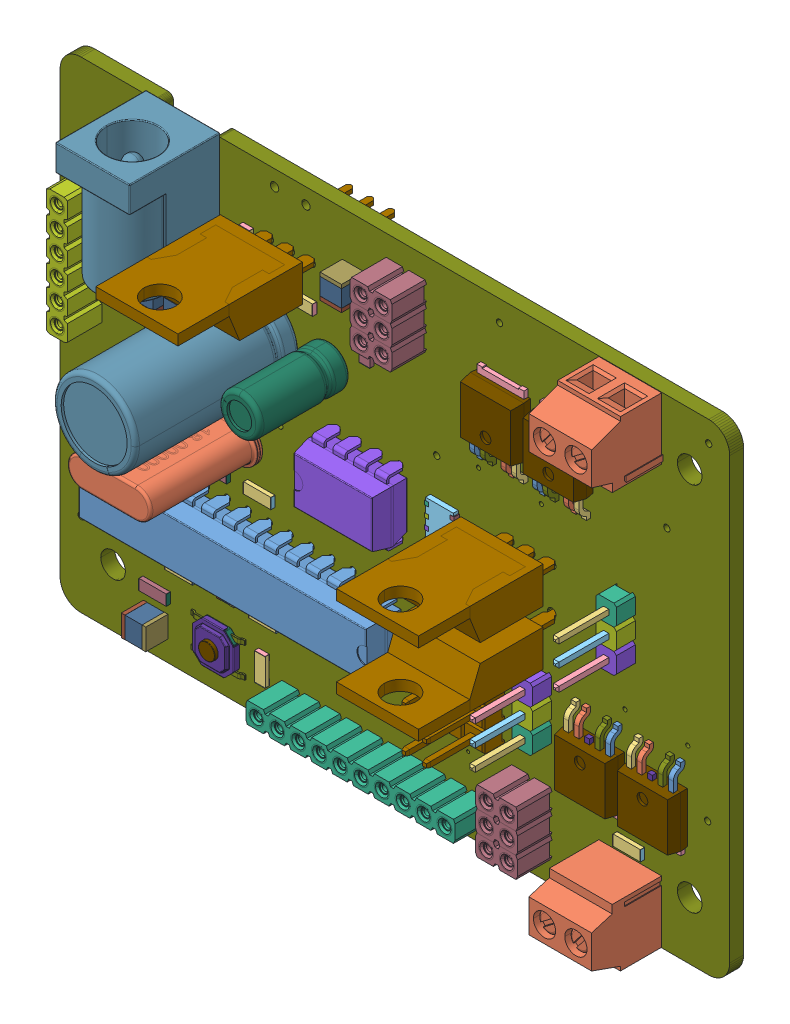
SolidWorks assembly Scheme_ver2, configuration По умолчанию. Lengths in mm.
Overall size (81.28 59.4 30.01).
257 component instances, 52 part files, 0 mates.
Components (placement in the parent):
- Scheme_ver2.STEP-1: Scheme_ver2.STEP [По умолчанию] at origin size (81.28 59.4 30.01)
  - U1.STEP-1: U1.STEP [По умолчанию] at (29.21 20.955 0.8452) x (-1 0 0) z (0 0 1) size (35.56 7.92 7.75)
    - Open CASCADE STEP translator 6.8 2.2.1.STEP-1: Open CASCADE STEP translator 6.8 2.2.1.STEP [По умолчанию] at origin size (35.56 7.92 7.75)
      - Body_1.STEP-1: Body_1.STEP [По умолчанию] at (16.5 3.8 0) x (0 1 0) z (1 0 0) size (7.92 7.75 35.56)
  - Y1.STEP-1: Y1.STEP [По умолчанию] at (10.16 27.94 0.8452) x (-1 0 0) z (0 0 1) size (11 4.5 15.2)
    - Open CASCADE STEP translator 6.8 2.3.1.STEP-1: Open CASCADE STEP translator 6.8 2.3.1.STEP [По умолчанию] at origin size (11 4.5 15.2)
      - Body_1-0.STEP-1: Body_1-0.STEP [По умолчанию] at (2.5 0 0) x (1 0 0) z (0 -1 0) size (11 15.2 4.5)
  - C6.STEP-1: C6.STEP [По умолчанию] at (6.35 31.7754 0.8452) x (0 1 0) z (0 0 1) size (3.35 1.3 0.55)
    - Open CASCADE STEP translator 6.8 2.4.1.STEP-1: Open CASCADE STEP translator 6.8 2.4.1.STEP [По умолчанию] at origin size (3.35 1.3 0.55)
      - Body_1-1.STEP-1: Body_1-1.STEP [По умолчанию] at origin size (3.3 1.3 0.48)
      - Pin_1.STEP-1: Pin_1.STEP [По умолчанию] at (0.5588 0 0) x (-1 0 0) z (0 0 1) size (0.76 1.27 0.55)
      - Pin_2.STEP-1: Pin_2.STEP [По умолчанию] at origin size (0.76 1.27 0.55)
  - C7.STEP-1: C7.STEP [По умолчанию] at (8.89 31.7754 0.8452) x (0 1 0) z (0 0 1) size (3.35 1.3 0.55)
    - Open CASCADE STEP translator 6.8 2.4.1.STEP-1: Open CASCADE STEP translator 6.8 2.4.1.STEP [По умолчанию] at origin size (3.35 1.3 0.55)
      - Body_1-1.STEP-1: Body_1-1.STEP [По умолчанию] at origin size (3.3 1.3 0.48)
      - Pin_1.STEP-1: Pin_1.STEP [По умолчанию] at (0.5588 0 0) x (-1 0 0) z (0 0 1) size (0.76 1.27 0.55)
      - Pin_2.STEP-1: Pin_2.STEP [По умолчанию] at origin size (0.76 1.27 0.55)
  - J1.STEP-1: J1.STEP [По умолчанию] at (16.51 3.81 0.8452) size (25.4 2.54 7.37)
    - Open CASCADE STEP translator 6.8 2.6.1.STEP-1: Open CASCADE STEP translator 6.8 2.6.1.STEP [По умолчанию] at origin size (25.4 2.54 7.37)
      - Body_1-2.STEP-1: Body_1-2.STEP [По умолчанию] at (11.5 0 0) x (1 0 0) z (0 -1 0) size (25.4 7.37 2.54)
  - J2.STEP-1: J2.STEP [По умолчанию] at (-7.62 45.72 0.8452) x (0 -1 0) z (0 0 1) size (15.24 2.54 7.37)
    - Open CASCADE STEP translator 6.8 2.7.1.STEP-1: Open CASCADE STEP translator 6.8 2.7.1.STEP [По умолчанию] at origin size (15.24 2.54 7.37)
      - Body_1-3.STEP-1: Body_1-3.STEP [По умолчанию] at (6.5 0 0) x (1 0 0) z (0 -1 0) size (15.24 7.37 2.54)
  - U2.STEP-1: U2.STEP [По умолчанию] at (22.225 27.305 0.8452) size (10.16 7.92 7.75)
    - Open CASCADE STEP translator 6.8 2.8.1.STEP-1: Open CASCADE STEP translator 6.8 2.8.1.STEP [По умолчанию] at origin size (10.16 7.92 7.75)
      - Body_1-4.STEP-1: Body_1-4.STEP [По умолчанию] at (3.9 4 0) x (0 1 0) z (1 0 0) size (7.92 7.75 10.16)
  - VT1.STEP-1: VT1.STEP [По умолчанию] at (45.72 33.655 0.8452) size (9.97 4.45 28.62)
    - Open CASCADE STEP translator 6.8 2.9.1.STEP-1: Open CASCADE STEP translator 6.8 2.9.1.STEP [По умолчанию] at origin size (9.97 4.45 28.62)
      - Body_1-5.STEP-1: Body_1-5.STEP [По умолчанию] at (0 3 3.5) x (1 0 0) z (0 -1 0) size (9.97 28.62 4.45)
  - VT2.STEP-1: VT2.STEP [По умолчанию] at (45.72 28.575 0.8452) x (-1 0 0) z (0 0 1) size (9.97 4.45 28.62)
    - Open CASCADE STEP translator 6.8 2.10.1.STEP-1: Open CASCADE STEP translator 6.8 2.10.1.STEP [По умолчанию] at origin size (9.97 4.45 28.62)
      - Body_1-5.STEP-1: Body_1-5.STEP [По умолчанию] at (0 3 3.5) x (1 0 0) z (0 -1 0) size (9.97 28.62 4.45)
  - D2.STEP-1: D2.STEP [По умолчанию] at (1.63 3.81 0.8452) x (-1 0 0) z (0 0 1) size (2.97 2.6 2.7)
    - Open CASCADE STEP translator 6.8 2.11.1.STEP-1: Open CASCADE STEP translator 6.8 2.11.1.STEP [По умолчанию] at origin size (2.97 2.6 2.7)
      - Body_1-6.STEP-1: Body_1-6.STEP [По умолчанию] at origin size (2.6 2.58 2.68)
      - Pin_1-7.STEP-1: Pin_1-7.STEP [По умолчанию] at origin size (0.45 2.6 2.7)
      - Pin_2-8.STEP-1: Pin_2-8.STEP [По умолчанию] at (0.376 0 0) x (-1 0 0) z (0 0 1) size (0.45 2.6 2.7)
  - R3.STEP-1: R3.STEP [По умолчанию] at (-1.27 6.985 0.8452) size (3.35 1.3 0.55)
    - Open CASCADE STEP translator 6.8 2.12.1.STEP-1: Open CASCADE STEP translator 6.8 2.12.1.STEP [По умолчанию] at origin size (3.35 1.3 0.55)
      - Body_1-9.STEP-1: Body_1-9.STEP [По умолчанию] at origin size (3.3 1.3 0.48)
      - Pin_1-10.STEP-1: Pin_1-10.STEP [По умолчанию] at (0.5588 0 0) x (-1 0 0) z (0 0 1) size (0.76 1.27 0.55)
      - Pin_2-11.STEP-1: Pin_2-11.STEP [По умолчанию] at origin size (0.76 1.27 0.55)
  - C2.STEP-1: C2.STEP [По умолчанию] at (11.43 50.8 0.8452) x (0 -1 0) z (0 0 1) size (3.35 1.3 0.55)
    - Open CASCADE STEP translator 6.8 2.4.1.STEP-1: Open CASCADE STEP translator 6.8 2.4.1.STEP [По умолчанию] at origin size (3.35 1.3 0.55)
      - Body_1-1.STEP-1: Body_1-1.STEP [По умолчанию] at origin size (3.3 1.3 0.48)
      - Pin_1.STEP-1: Pin_1.STEP [По умолчанию] at (0.5588 0 0) x (-1 0 0) z (0 0 1) size (0.76 1.27 0.55)
      - Pin_2.STEP-1: Pin_2.STEP [По умолчанию] at origin size (0.76 1.27 0.55)
  - DA1.STEP-1: DA1.STEP [По умолчанию] at (16.51 50.8 0.8452) size (9.97 4.45 28.62)
    - Open CASCADE STEP translator 6.8 2.14.1.STEP-1: Open CASCADE STEP translator 6.8 2.14.1.STEP [По умолчанию] at origin size (9.97 4.45 28.62)
      - Body_1-5.STEP-1: Body_1-5.STEP [По умолчанию] at (0 3 3.5) x (1 0 0) z (0 -1 0) size (9.97 28.62 4.45)
  - C3.STEP-1: C3.STEP [По умолчанию] at (19.644 46.355 0.8452) x (-1 0 0) z (0 0 1) size (3.35 1.3 0.55)
    - Open CASCADE STEP translator 6.8 2.4.1.STEP-1: Open CASCADE STEP translator 6.8 2.4.1.STEP [По умолчанию] at origin size (3.35 1.3 0.55)
      - Body_1-1.STEP-1: Body_1-1.STEP [По умолчанию] at origin size (3.3 1.3 0.48)
      - Pin_1.STEP-1: Pin_1.STEP [По умолчанию] at (0.5588 0 0) x (-1 0 0) z (0 0 1) size (0.76 1.27 0.55)
      - Pin_2.STEP-1: Pin_2.STEP [По умолчанию] at origin size (0.76 1.27 0.55)
  - C5.STEP-1: C5.STEP [По умолчанию] at (11.43 23.495 0.8452) size (3.35 1.3 0.55)
    - Open CASCADE STEP translator 6.8 2.4.1.STEP-1: Open CASCADE STEP translator 6.8 2.4.1.STEP [По умолчанию] at origin size (3.35 1.3 0.55)
      - Body_1-1.STEP-1: Body_1-1.STEP [По умолчанию] at origin size (3.3 1.3 0.48)
      - Pin_1.STEP-1: Pin_1.STEP [По умолчанию] at (0.5588 0 0) x (-1 0 0) z (0 0 1) size (0.76 1.27 0.55)
      - Pin_2.STEP-1: Pin_2.STEP [По умолчанию] at origin size (0.76 1.27 0.55)
  - Q2.STEP-1: Q2.STEP [По умолчанию] at (39.9815 41.3198 0.8452) size (6.5 9.8 2.31)
    - Open CASCADE STEP translator 6.8 2.17.1.STEP-1: Open CASCADE STEP translator 6.8 2.17.1.STEP [По умолчанию] at origin size (6.5 9.8 2.31)
      - Body_1-12.STEP-1: Body_1-12.STEP [По умолчанию] at (2.4 5.35 0) size (6.5 9.8 2.31)
        - Scheme_ver2-prt15.STEP-1: Scheme_ver2-prt15.STEP [По умолчанию] at origin size (0.6 3 1.4)
        - Scheme_ver2-prt16.STEP-1: Scheme_ver2-prt16.STEP [По умолчанию] at (0.13 0 0) size (0.6 0.85 0.5)
        - Scheme_ver2-prt17.STEP-1: Scheme_ver2-prt17.STEP [По умолчанию] at (0.129 0.01 -0.0028) x (0.999999 0 -0.001062) z (0.001062 0 0.999999) size (6.5 6.22 2.3)
        - Scheme_ver2-prt18.STEP-1: Scheme_ver2-prt18.STEP [По умолчанию] at (-0.13 0 0) size (0.6 3 1.4)
        - Scheme_ver2-prt19.STEP-1: Scheme_ver2-prt19.STEP [По умолчанию] at (0.26 0 0) size (0.6 3 1.4)
        - Scheme_ver2-prt20.STEP-1: Scheme_ver2-prt20.STEP [По умолчанию] at (0.39 0 0) size (0.6 3 1.4)
        - Scheme_ver2-prt21.STEP-1: Scheme_ver2-prt21.STEP [По умолчанию] at (0.129 -0.1 -0.0028) x (0.999999 0 -0.001062) z (0.001062 0 0.999999) size (5.7 5.2 0.5)
  - Q1.STEP-1: Q1.STEP [По умолчанию] at (47.6015 41.3198 0.8452) size (6.5 9.8 2.31)
    - Open CASCADE STEP translator 6.8 2.18.1.STEP-1: Open CASCADE STEP translator 6.8 2.18.1.STEP [По умолчанию] at origin size (6.5 9.8 2.31)
      - Body_1-12.STEP-1: Body_1-12.STEP [По умолчанию] at (2.4 5.35 0) size (6.5 9.8 2.31)
        - Scheme_ver2-prt15.STEP-1: Scheme_ver2-prt15.STEP [По умолчанию] at origin size (0.6 3 1.4)
        - Scheme_ver2-prt16.STEP-1: Scheme_ver2-prt16.STEP [По умолчанию] at (0.13 0 0) size (0.6 0.85 0.5)
        - Scheme_ver2-prt17.STEP-1: Scheme_ver2-prt17.STEP [По умолчанию] at (0.129 0.01 -0.0028) x (0.999999 0 -0.001062) z (0.001062 0 0.999999) size (6.5 6.22 2.3)
        - Scheme_ver2-prt18.STEP-1: Scheme_ver2-prt18.STEP [По умолчанию] at (-0.13 0 0) size (0.6 3 1.4)
        - Scheme_ver2-prt19.STEP-1: Scheme_ver2-prt19.STEP [По умолчанию] at (0.26 0 0) size (0.6 3 1.4)
        - Scheme_ver2-prt20.STEP-1: Scheme_ver2-prt20.STEP [По умолчанию] at (0.39 0 0) size (0.6 3 1.4)
        - Scheme_ver2-prt21.STEP-1: Scheme_ver2-prt21.STEP [По умолчанию] at (0.129 -0.1 -0.0028) x (0.999999 0 -0.001062) z (0.001062 0 0.999999) size (5.7 5.2 0.5)
  - D1.STEP-1: D1.STEP [По умолчанию] at (24.13 52.98 0.8452) x (0 -1 0) z (0 0 1) size (2.97 2.6 2.7)
    - Open CASCADE STEP translator 6.8 2.11.1.STEP-1: Open CASCADE STEP translator 6.8 2.11.1.STEP [По умолчанию] at origin size (2.97 2.6 2.7)
      - Body_1-6.STEP-1: Body_1-6.STEP [По умолчанию] at origin size (2.6 2.58 2.68)
      - Pin_1-7.STEP-1: Pin_1-7.STEP [По умолчанию] at origin size (0.45 2.6 2.7)
      - Pin_2-8.STEP-1: Pin_2-8.STEP [По умолчанию] at (0.376 0 0) x (-1 0 0) z (0 0 1) size (0.45 2.6 2.7)
  - R1.STEP-1: R1.STEP [По умолчанию] at (26.035 43.815 0.8452) x (0 1 0) z (0 0 1) size (3.35 1.3 0.55)
    - Open CASCADE STEP translator 6.8 2.12.1.STEP-1: Open CASCADE STEP translator 6.8 2.12.1.STEP [По умолчанию] at origin size (3.35 1.3 0.55)
      - Body_1-9.STEP-1: Body_1-9.STEP [По умолчанию] at origin size (3.3 1.3 0.48)
      - Pin_1-10.STEP-1: Pin_1-10.STEP [По умолчанию] at (0.5588 0 0) x (-1 0 0) z (0 0 1) size (0.76 1.27 0.55)
      - Pin_2-11.STEP-1: Pin_2-11.STEP [По умолчанию] at origin size (0.76 1.27 0.55)
  - Q4.STEP-1: Q4.STEP [По умолчанию] at (64.095 20.67 0.8452) x (-1 0 0) z (0 0 1) size (6.5 9.8 2.31)
    - Open CASCADE STEP translator 6.8 2.21.1.STEP-1: Open CASCADE STEP translator 6.8 2.21.1.STEP [По умолчанию] at origin size (6.5 9.8 2.31)
      - Body_1-12.STEP-1: Body_1-12.STEP [По умолчанию] at (2.4 5.35 0) size (6.5 9.8 2.31)
        - Scheme_ver2-prt15.STEP-1: Scheme_ver2-prt15.STEP [По умолчанию] at origin size (0.6 3 1.4)
        - Scheme_ver2-prt16.STEP-1: Scheme_ver2-prt16.STEP [По умолчанию] at (0.13 0 0) size (0.6 0.85 0.5)
        - Scheme_ver2-prt17.STEP-1: Scheme_ver2-prt17.STEP [По умолчанию] at (0.129 0.01 -0.0028) x (0.999999 0 -0.001062) z (0.001062 0 0.999999) size (6.5 6.22 2.3)
        - Scheme_ver2-prt18.STEP-1: Scheme_ver2-prt18.STEP [По умолчанию] at (-0.13 0 0) size (0.6 3 1.4)
        - Scheme_ver2-prt19.STEP-1: Scheme_ver2-prt19.STEP [По умолчанию] at (0.26 0 0) size (0.6 3 1.4)
        - Scheme_ver2-prt20.STEP-1: Scheme_ver2-prt20.STEP [По умолчанию] at (0.39 0 0) size (0.6 3 1.4)
        - Scheme_ver2-prt21.STEP-1: Scheme_ver2-prt21.STEP [По умолчанию] at (0.129 -0.1 -0.0028) x (0.999999 0 -0.001062) z (0.001062 0 0.999999) size (5.7 5.2 0.5)
  - Q3.STEP-1: Q3.STEP [По умолчанию] at (56.475 20.67 0.8452) x (-1 0 0) z (0 0 1) size (6.5 9.8 2.31)
    - Open CASCADE STEP translator 6.8 2.22.1.STEP-1: Open CASCADE STEP translator 6.8 2.22.1.STEP [По умолчанию] at origin size (6.5 9.8 2.31)
      - Body_1-12.STEP-1: Body_1-12.STEP [По умолчанию] at (2.4 5.35 0) size (6.5 9.8 2.31)
        - Scheme_ver2-prt15.STEP-1: Scheme_ver2-prt15.STEP [По умолчанию] at origin size (0.6 3 1.4)
        - Scheme_ver2-prt16.STEP-1: Scheme_ver2-prt16.STEP [По умолчанию] at (0.13 0 0) size (0.6 0.85 0.5)
        - Scheme_ver2-prt17.STEP-1: Scheme_ver2-prt17.STEP [По умолчанию] at (0.129 0.01 -0.0028) x (0.999999 0 -0.001062) z (0.001062 0 0.999999) size (6.5 6.22 2.3)
        - Scheme_ver2-prt18.STEP-1: Scheme_ver2-prt18.STEP [По умолчанию] at (-0.13 0 0) size (0.6 3 1.4)
        - Scheme_ver2-prt19.STEP-1: Scheme_ver2-prt19.STEP [По умолчанию] at (0.26 0 0) size (0.6 3 1.4)
        - Scheme_ver2-prt20.STEP-1: Scheme_ver2-prt20.STEP [По умолчанию] at (0.39 0 0) size (0.6 3 1.4)
        - Scheme_ver2-prt21.STEP-1: Scheme_ver2-prt21.STEP [По умолчанию] at (0.129 -0.1 -0.0028) x (0.999999 0 -0.001062) z (0.001062 0 0.999999) size (5.7 5.2 0.5)
  - C12.STEP-1: C12.STEP [По умолчанию] at (56.2864 8.89 0.8452) size (3.35 1.3 0.55)
    - Open CASCADE STEP translator 6.8 2.4.1.STEP-1: Open CASCADE STEP translator 6.8 2.4.1.STEP [По умолчанию] at origin size (3.35 1.3 0.55)
      - Body_1-1.STEP-1: Body_1-1.STEP [По умолчанию] at origin size (3.3 1.3 0.48)
      - Pin_1.STEP-1: Pin_1.STEP [По умолчанию] at (0.5588 0 0) x (-1 0 0) z (0 0 1) size (0.76 1.27 0.55)
      - Pin_2.STEP-1: Pin_2.STEP [По умолчанию] at origin size (0.76 1.27 0.55)
  - C11.STEP-1: C11.STEP [По умолчанию] at (56.261 49.53 0.8452) size (3.35 1.3 0.55)
    - Open CASCADE STEP translator 6.8 2.4.1.STEP-1: Open CASCADE STEP translator 6.8 2.4.1.STEP [По умолчанию] at origin size (3.35 1.3 0.55)
      - Body_1-1.STEP-1: Body_1-1.STEP [По умолчанию] at origin size (3.3 1.3 0.48)
      - Pin_1.STEP-1: Pin_1.STEP [По умолчанию] at (0.5588 0 0) x (-1 0 0) z (0 0 1) size (0.76 1.27 0.55)
      - Pin_2.STEP-1: Pin_2.STEP [По умолчанию] at origin size (0.76 1.27 0.55)
  - RN1.STEP-1: RN1.STEP [По умолчанию] at (33.68 31.75 0.8452) size (3.6 5.11 0.63)
    - Open CASCADE STEP translator 6.8 2.25.1.STEP-1: Open CASCADE STEP translator 6.8 2.25.1.STEP [По умолчанию] at origin size (3.6 5.11 0.63)
      - Body_1-13.STEP-1: Body_1-13.STEP [По умолчанию] at origin size (3.38 5.11 0.61)
      - Pin_1-14.STEP-1: Pin_1-14.STEP [По умолчанию] at (0 2.64 0) x (-1 0 0) z (0 0 1) size (0.5 0.5 0.63)
      - Pin_2-15.STEP-1: Pin_2-15.STEP [По умолчанию] x (-1 0 0) z (0 0 1) size (0.5 0.5 0.63)
      - Pin_3.STEP-1: Pin_3.STEP [По умолчанию] at (0 -2.54 0) x (-1 0 0) z (0 0 1) size (0.5 0.5 0.63)
      - Pin_4.STEP-1: Pin_4.STEP [По умолчанию] at (0 -5.18 0) x (-1 0 0) z (0 0 1) size (0.5 0.5 0.63)
      - Pin_5.STEP-1: Pin_5.STEP [По умолчанию] at origin size (0.5 0.5 0.63)
      - Pin_6.STEP-1: Pin_6.STEP [По умолчанию] at origin size (0.5 0.5 0.63)
      - Pin_7.STEP-1: Pin_7.STEP [По умолчанию] at origin size (0.5 0.5 0.63)
      - Pin_8.STEP-1: Pin_8.STEP [По умолчанию] at origin size (0.5 0.5 0.63)
  - Open CASCADE STEP translator 6.8 2.26.STEP-1: Open CASCADE STEP translator 6.8 2.26.STEP [По умолчанию] at (4 52 0.8452) size (9.01 14.01 14.5)
    - Open CASCADE STEP translator 6.8 2.26.1.STEP-1: Open CASCADE STEP translator 6.8 2.26.1.STEP [По умолчанию] at origin size (9.01 14.01 14.5)
      - Body_1-16.STEP-1: Body_1-16.STEP [По умолчанию] at (0 7.4 6) x (-1 0 0) z (0 1 0) size (9.01 14.5 14.01)
  - RESET.STEP-1: RESET.STEP [По умолчанию] at (10.795 3.175 0.8452) size (6.55 5.45 1.56)
    - Open CASCADE STEP translator 6.8 2.27.1.STEP-1: Open CASCADE STEP translator 6.8 2.27.1.STEP [По умолчанию] at origin size (6.55 5.45 1.56)
      - Body_1-1-17.STEP-1: Body_1-1-17.STEP [По умолчанию] at (-2.9 1.9 0) x (1 0 0) z (0 -1 0) size (6.55 1.56 5.45)
        - Scheme_ver2-prt32.STEP-1: Scheme_ver2-prt32.STEP [По умолчанию] at origin size (4.85 0.7 4.85)
        - Scheme_ver2-prt33.STEP-1: Scheme_ver2-prt33.STEP [По умолчанию] at (0 -0.01 0) size (6.55 0.42 4.2)
        - Scheme_ver2-prt34.STEP-1: Scheme_ver2-prt34.STEP [По умолчанию] at (0 0.7 0) size (5.05 1.15 5.05)
        - Scheme_ver2-prt35.STEP-1: Scheme_ver2-prt35.STEP [По умолчанию] at (0 1.05 0) size (2.87 0.7 2.87)
        - Scheme_ver2-prt36.STEP-1: Scheme_ver2-prt36.STEP [По умолчанию] at (0 0.4172 0) x (0.87225 0 -0.489061) z (0.489061 0 0.87225) size (4 0.44 4)
  - M2.STEP-1: M2.STEP [По умолчанию] at (55.88 3.81 0.8452) size (7.81 7.5 12)
    - Open CASCADE STEP translator 6.8 2.28.1.STEP-1: Open CASCADE STEP translator 6.8 2.28.1.STEP [По умолчанию] at origin size (7.81 7.5 12)
      - Body_1-18.STEP-1: Body_1-18.STEP [По умолчанию] at (1.9 0 0) x (-1 0 0) z (0 0 1) size (7.81 7.5 12)
  - M1.STEP-1: M1.STEP [По умолчанию] at (59.69 54.61 0.8452) x (-1 0 0) z (0 0 1) size (7.81 7.5 12)
    - Open CASCADE STEP translator 6.8 2.29.1.STEP-1: Open CASCADE STEP translator 6.8 2.29.1.STEP [По умолчанию] at origin size (7.81 7.5 12)
      - Body_1-18.STEP-1: Body_1-18.STEP [По умолчанию] at (1.9 0 0) x (-1 0 0) z (0 0 1) size (7.81 7.5 12)
  - PWR_MOTOR.STEP-1: PWR_MOTOR.STEP [По умолчанию] at (57.15 34.29 0.8452) size (2.49 7.62 11.54)
    - Open CASCADE STEP translator 6.8 2.30.1.STEP-1: Open CASCADE STEP translator 6.8 2.30.1.STEP [По умолчанию] at origin size (2.49 7.62 11.54)
      - Body_1-2-19.STEP-1: Body_1-2-19.STEP [По умолчанию] at (0 -5 0) x (0 1 0) z (0 0 1) size (7.62 2.49 11.54)
        - Scheme_ver2-asm54.STEP-1: Scheme_ver2-asm54.STEP [По умолчанию] at origin size (5.72 0.64 11.54)
          - SOLID.STEP-1: SOLID.STEP [По умолчанию] at origin size (0.64 0.64 11.54)
          - SOLID-20.STEP-1: SOLID-20.STEP [По умолчанию] at origin size (0.64 0.64 11.54)
          - SOLID-21.STEP-1: SOLID-21.STEP [По умолчанию] at origin size (0.64 0.64 11.54)
        - Scheme_ver2-asm55.STEP-1: Scheme_ver2-asm55.STEP [По умолчанию] at origin size (7.62 2.49 2.29)
          - SOLID-22.STEP-1: SOLID-22.STEP [По умолчанию] at origin size (2.54 2.49 2.29)
          - SOLID-23.STEP-1: SOLID-23.STEP [По умолчанию] at origin size (2.54 2.49 2.29)
          - SOLID-24.STEP-1: SOLID-24.STEP [По умолчанию] at origin size (2.54 2.49 2.29)
  - ICSP.STEP-1: ICSP.STEP [По умолчанию] at (38.735 18.415 0.8452) size (5.08 7.62 10.98)
    - Open CASCADE STEP translator 6.8 2.31.1.STEP-1: Open CASCADE STEP translator 6.8 2.31.1.STEP [По умолчанию] at origin size (5.08 7.62 10.98)
      - Body_1-3-25.STEP-1: Body_1-3-25.STEP [По умолчанию] at (1.25 -2.6 0) x (1 0 0) z (0 -1 0) size (5.08 10.98 7.62)
        - Scheme_ver2-asm59.STEP-1: Scheme_ver2-asm59.STEP [По умолчанию] at (-5.6755 -6.84 9.2218) size (5.08 10.98 2.54)
          - Scheme_ver2-prt44.STEP-1: Scheme_ver2-prt44.STEP [По умолчанию] at (4.4052 8.1155 -11.7669) size (2.54 10.98 2.54)
          - Scheme_ver2-prt44.STEP-2: Scheme_ver2-prt44.STEP [По умолчанию] at (6.9452 8.1155 -11.7669) size (2.54 10.98 2.54)
        - Scheme_ver2-asm60.STEP-1: Scheme_ver2-asm60.STEP [По умолчанию] at (-5.6755 -6.84 11.7618) size (5.08 10.98 2.54)
          - Scheme_ver2-prt44.STEP-1: Scheme_ver2-prt44.STEP [По умолчанию] at (4.4052 8.1155 -11.7669) size (2.54 10.98 2.54)
          - Scheme_ver2-prt44.STEP-2: Scheme_ver2-prt44.STEP [По умолчанию] at (6.9452 8.1155 -11.7669) size (2.54 10.98 2.54)
        - Scheme_ver2-asm61.STEP-1: Scheme_ver2-asm61.STEP [По умолчанию] at (-5.6755 -6.84 14.3018) size (5.08 10.98 2.54)
          - Scheme_ver2-prt44.STEP-1: Scheme_ver2-prt44.STEP [По умолчанию] at (4.4052 8.1155 -11.7669) size (2.54 10.98 2.54)
          - Scheme_ver2-prt44.STEP-2: Scheme_ver2-prt44.STEP [По умолчанию] at (6.9452 8.1155 -11.7669) size (2.54 10.98 2.54)
  - R5.STEP-1: R5.STEP [По умолчанию] at (0 34.925 0.8452) x (0 -1 0) z (0 0 1) size (3.35 1.3 0.55)
    - Open CASCADE STEP translator 6.8 2.12.1.STEP-1: Open CASCADE STEP translator 6.8 2.12.1.STEP [По умолчанию] at origin size (3.35 1.3 0.55)
      - Body_1-9.STEP-1: Body_1-9.STEP [По умолчанию] at origin size (3.3 1.3 0.48)
      - Pin_1-10.STEP-1: Pin_1-10.STEP [По умолчанию] at (0.5588 0 0) x (-1 0 0) z (0 0 1) size (0.76 1.27 0.55)
      - Pin_2-11.STEP-1: Pin_2-11.STEP [По умолчанию] at origin size (0.76 1.27 0.55)
  - C9.STEP-1: C9.STEP [По умолчанию] at (12.065 10.795 0.8452) size (3.35 1.3 0.55)
    - Open CASCADE STEP translator 6.8 2.4.1.STEP-1: Open CASCADE STEP translator 6.8 2.4.1.STEP [По умолчанию] at origin size (3.35 1.3 0.55)
      - Body_1-1.STEP-1: Body_1-1.STEP [По умолчанию] at origin size (3.3 1.3 0.48)
      - Pin_1.STEP-1: Pin_1.STEP [По умолчанию] at (0.5588 0 0) x (-1 0 0) z (0 0 1) size (0.76 1.27 0.55)
      - Pin_2.STEP-1: Pin_2.STEP [По умолчанию] at origin size (0.76 1.27 0.55)
  - R2.STEP-1: R2.STEP [По умолчанию] at (6.0452 23.495 0.8452) size (3.35 1.3 0.55)
    - Open CASCADE STEP translator 6.8 2.12.1.STEP-1: Open CASCADE STEP translator 6.8 2.12.1.STEP [По умолчанию] at origin size (3.35 1.3 0.55)
      - Body_1-9.STEP-1: Body_1-9.STEP [По умолчанию] at origin size (3.3 1.3 0.48)
      - Pin_1-10.STEP-1: Pin_1-10.STEP [По умолчанию] at (0.5588 0 0) x (-1 0 0) z (0 0 1) size (0.76 1.27 0.55)
      - Pin_2-11.STEP-1: Pin_2-11.STEP [По умолчанию] at origin size (0.76 1.27 0.55)
  - JP1.STEP-1: JP1.STEP [По умолчанию] at (46.99 15.875 0.8452) x (-1 0 0) z (0 0 1) size (2.49 7.62 11.54)
    - Open CASCADE STEP translator 6.8 2.35.1.STEP-1: Open CASCADE STEP translator 6.8 2.35.1.STEP [По умолчанию] at origin size (2.49 7.62 11.54)
      - Body_1-2-19.STEP-1: Body_1-2-19.STEP [По умолчанию] at (0 -5 0) x (0 1 0) z (0 0 1) size (7.62 2.49 11.54)
        - Scheme_ver2-asm54.STEP-1: Scheme_ver2-asm54.STEP [По умолчанию] at origin size (5.72 0.64 11.54)
          - SOLID.STEP-1: SOLID.STEP [По умолчанию] at origin size (0.64 0.64 11.54)
          - SOLID-20.STEP-1: SOLID-20.STEP [По умолчанию] at origin size (0.64 0.64 11.54)
          - SOLID-21.STEP-1: SOLID-21.STEP [По умолчанию] at origin size (0.64 0.64 11.54)
        - Scheme_ver2-asm55.STEP-1: Scheme_ver2-asm55.STEP [По умолчанию] at origin size (7.62 2.49 2.29)
          - SOLID-22.STEP-1: SOLID-22.STEP [По умолчанию] at origin size (2.54 2.49 2.29)
          - SOLID-23.STEP-1: SOLID-23.STEP [По умолчанию] at origin size (2.54 2.49 2.29)
          - SOLID-24.STEP-1: SOLID-24.STEP [По умолчанию] at origin size (2.54 2.49 2.29)
  - C8.STEP-1: C8.STEP [По умолчанию] at (1.905 10.795 0.8452) size (3.35 1.3 0.55)
    - Open CASCADE STEP translator 6.8 2.4.1.STEP-1: Open CASCADE STEP translator 6.8 2.4.1.STEP [По умолчанию] at origin size (3.35 1.3 0.55)
      - Body_1-1.STEP-1: Body_1-1.STEP [По умолчанию] at origin size (3.3 1.3 0.48)
      - Pin_1.STEP-1: Pin_1.STEP [По умолчанию] at (0.5588 0 0) x (-1 0 0) z (0 0 1) size (0.76 1.27 0.55)
      - Pin_2.STEP-1: Pin_2.STEP [По умолчанию] at origin size (0.76 1.27 0.55)
  - L1.STEP-1: L1.STEP [По умолчанию] at (8.0838 10.7934 0.8452) size (2.08 1.02 0.51)
    - Open CASCADE STEP translator 6.8 2.37.1.STEP-1: Open CASCADE STEP translator 6.8 2.37.1.STEP [По умолчанию] at origin size (2.08 1.02 0.51)
      - Body_1-26.STEP-1: Body_1-26.STEP [По умолчанию] at origin size (1.14 0.99 0.46)
      - Pin_1-27.STEP-1: Pin_1-27.STEP [По умолчанию] at origin size (0.51 1.02 0.51)
      - Pin_2-28.STEP-1: Pin_2-28.STEP [По умолчанию] at (3.6444 0.0032 0) x (-1 0 0) z (0 0 1) size (0.51 1.02 0.51)
  - C10.STEP-1: C10.STEP [По умолчанию] at (13.335 6.985 0.8452) x (0 -1 0) z (0 0 1) size (3.35 1.3 0.55)
    - Open CASCADE STEP translator 6.8 2.4.1.STEP-1: Open CASCADE STEP translator 6.8 2.4.1.STEP [По умолчанию] at origin size (3.35 1.3 0.55)
      - Body_1-1.STEP-1: Body_1-1.STEP [По умолчанию] at origin size (3.3 1.3 0.48)
      - Pin_1.STEP-1: Pin_1.STEP [По умолчанию] at (0.5588 0 0) x (-1 0 0) z (0 0 1) size (0.76 1.27 0.55)
      - Pin_2.STEP-1: Pin_2.STEP [По умолчанию] at origin size (0.76 1.27 0.55)
  - Open CASCADE STEP translator 6.8 2.39.STEP-1: Open CASCADE STEP translator 6.8 2.39.STEP [По умолчанию] at (44.45 3.81 0.8452) size (5.08 2.54 7.37)
    - Open CASCADE STEP translator 6.8 2.39.1.STEP-1: Open CASCADE STEP translator 6.8 2.39.1.STEP [По умолчанию] at origin size (5.08 2.54 7.37)
      - Body_1-29.STEP-1: Body_1-29.STEP [По умолчанию] at (1.3 0 0) x (1 0 0) z (0 -1 0) size (5.08 7.37 2.54)
  - Open CASCADE STEP translator 6.8 2.40.STEP-1: Open CASCADE STEP translator 6.8 2.40.STEP [По умолчанию] at (44.45 6.35 0.8452) size (5.08 2.54 7.37)
    - Open CASCADE STEP translator 6.8 2.40.1.STEP-1: Open CASCADE STEP translator 6.8 2.40.1.STEP [По умолчанию] at origin size (5.08 2.54 7.37)
      - Body_1-29.STEP-1: Body_1-29.STEP [По умолчанию] at (1.3 0 0) x (1 0 0) z (0 -1 0) size (5.08 7.37 2.54)
  - Open CASCADE STEP translator 6.8 2.41.STEP-1: Open CASCADE STEP translator 6.8 2.41.STEP [По умолчанию] at (44.45 8.89 0.8452) size (5.08 2.54 7.37)
    - Open CASCADE STEP translator 6.8 2.41.1.STEP-1: Open CASCADE STEP translator 6.8 2.41.1.STEP [По умолчанию] at origin size (5.08 2.54 7.37)
      - Body_1-29.STEP-1: Body_1-29.STEP [По умолчанию] at (1.3 0 0) x (1 0 0) z (0 -1 0) size (5.08 7.37 2.54)
  - Open CASCADE STEP translator 6.8 2.42.STEP-1: Open CASCADE STEP translator 6.8 2.42.STEP [По умолчанию] at (29.21 49.53 0.8452) size (5.08 2.54 7.37)
    - Open CASCADE STEP translator 6.8 2.42.1.STEP-1: Open CASCADE STEP translator 6.8 2.42.1.STEP [По умолчанию] at origin size (5.08 2.54 7.37)
      - Body_1-29.STEP-1: Body_1-29.STEP [По умолчанию] at (1.3 0 0) x (1 0 0) z (0 -1 0) size (5.08 7.37 2.54)
  - Open CASCADE STEP translator 6.8 2.43.STEP-1: Open CASCADE STEP translator 6.8 2.43.STEP [По умолчанию] at (29.21 52.07 0.8452) size (5.08 2.54 7.37)
    - Open CASCADE STEP translator 6.8 2.43.1.STEP-1: Open CASCADE STEP translator 6.8 2.43.1.STEP [По умолчанию] at origin size (5.08 2.54 7.37)
      - Body_1-29.STEP-1: Body_1-29.STEP [По умолчанию] at (1.3 0 0) x (1 0 0) z (0 -1 0) size (5.08 7.37 2.54)
  - Open CASCADE STEP translator 6.8 2.44.STEP-1: Open CASCADE STEP translator 6.8 2.44.STEP [По умолчанию] at (29.21 54.61 0.8452) size (5.08 2.54 7.37)
    - Open CASCADE STEP translator 6.8 2.44.1.STEP-1: Open CASCADE STEP translator 6.8 2.44.1.STEP [По умолчанию] at origin size (5.08 2.54 7.37)
      - Body_1-29.STEP-1: Body_1-29.STEP [По умолчанию] at (1.3 0 0) x (1 0 0) z (0 -1 0) size (5.08 7.37 2.54)
  - R6.STEP-1: R6.STEP [По умолчанию] at (2.54 34.925 0.8452) x (0 -1 0) z (0 0 1) size (3.35 1.3 0.55)
    - Open CASCADE STEP translator 6.8 2.12.1.STEP-1: Open CASCADE STEP translator 6.8 2.12.1.STEP [По умолчанию] at origin size (3.35 1.3 0.55)
      - Body_1-9.STEP-1: Body_1-9.STEP [По умолчанию] at origin size (3.3 1.3 0.48)
      - Pin_1-10.STEP-1: Pin_1-10.STEP [По умолчанию] at (0.5588 0 0) x (-1 0 0) z (0 0 1) size (0.76 1.27 0.55)
      - Pin_2-11.STEP-1: Pin_2-11.STEP [По умолчанию] at origin size (0.76 1.27 0.55)
  - D3.STEP-1: D3.STEP [По умолчанию] at (1.27 41.275 0.8452) x (0 -1 0) z (0 0 1) size (2.97 2.6 2.7)
    - Open CASCADE STEP translator 6.8 2.11.1.STEP-1: Open CASCADE STEP translator 6.8 2.11.1.STEP [По умолчанию] at origin size (2.97 2.6 2.7)
      - Body_1-6.STEP-1: Body_1-6.STEP [По умолчанию] at origin size (2.6 2.58 2.68)
      - Pin_1-7.STEP-1: Pin_1-7.STEP [По умолчанию] at origin size (0.45 2.6 2.7)
      - Pin_2-8.STEP-1: Pin_2-8.STEP [По умолчанию] at (0.376 0 0) x (-1 0 0) z (0 0 1) size (0.45 2.6 2.7)
  - D4.STEP-1: D4.STEP [По умолчанию] at (5.08 41.275 0.8452) x (0 -1 0) z (0 0 1) size (2.97 2.6 2.7)
    - Open CASCADE STEP translator 6.8 2.11.1.STEP-1: Open CASCADE STEP translator 6.8 2.11.1.STEP [По умолчанию] at origin size (2.97 2.6 2.7)
      - Body_1-6.STEP-1: Body_1-6.STEP [По умолчанию] at origin size (2.6 2.58 2.68)
      - Pin_1-7.STEP-1: Pin_1-7.STEP [По умолчанию] at origin size (0.45 2.6 2.7)
      - Pin_2-8.STEP-1: Pin_2-8.STEP [По умолчанию] at (0.376 0 0) x (-1 0 0) z (0 0 1) size (0.45 2.6 2.7)
  - C1.STEP-1: C1.STEP [По умолчанию] at (12.7 43.18 0.8452) x (0 1 0) z (0 0 1) size (10.01 10 22.71)
    - Open CASCADE STEP translator 6.8 2.48.1.STEP-1: Open CASCADE STEP translator 6.8 2.48.1.STEP [По умолчанию] at origin size (10.01 10 22.71)
      - Body_1-30.STEP-1: Body_1-30.STEP [По умолчанию] at (-2.6 0 0) x (-1 0 0) z (0 1 0) size (10.01 22.71 10)
  - C4.STEP-1: C4.STEP [По умолчанию] at (20.32 41.275 0.8452) size (5.01 5 13.71)
    - Open CASCADE STEP translator 6.8 2.49.1.STEP-1: Open CASCADE STEP translator 6.8 2.49.1.STEP [По умолчанию] at origin size (5.01 5 13.71)
      - Body_1-31.STEP-1: Body_1-31.STEP [По умолчанию] at (1 0 0) x (-1 0 0) z (0 1 0) size (5.01 13.71 5)
  - R4.STEP-1: R4.STEP [По умолчанию] at (33.02 12.065 0.8452) size (3.35 1.3 0.55)
    - Open CASCADE STEP translator 6.8 2.12.1.STEP-1: Open CASCADE STEP translator 6.8 2.12.1.STEP [По умолчанию] at origin size (3.35 1.3 0.55)
      - Body_1-9.STEP-1: Body_1-9.STEP [По умолчанию] at origin size (3.3 1.3 0.48)
      - Pin_1-10.STEP-1: Pin_1-10.STEP [По умолчанию] at (0.5588 0 0) x (-1 0 0) z (0 0 1) size (0.76 1.27 0.55)
      - Pin_2-11.STEP-1: Pin_2-11.STEP [По умолчанию] at origin size (0.76 1.27 0.55)
  - Layer_1.STEP-1: Layer_1.STEP [По умолчанию] at origin size (81.28 58.42 1.69)
